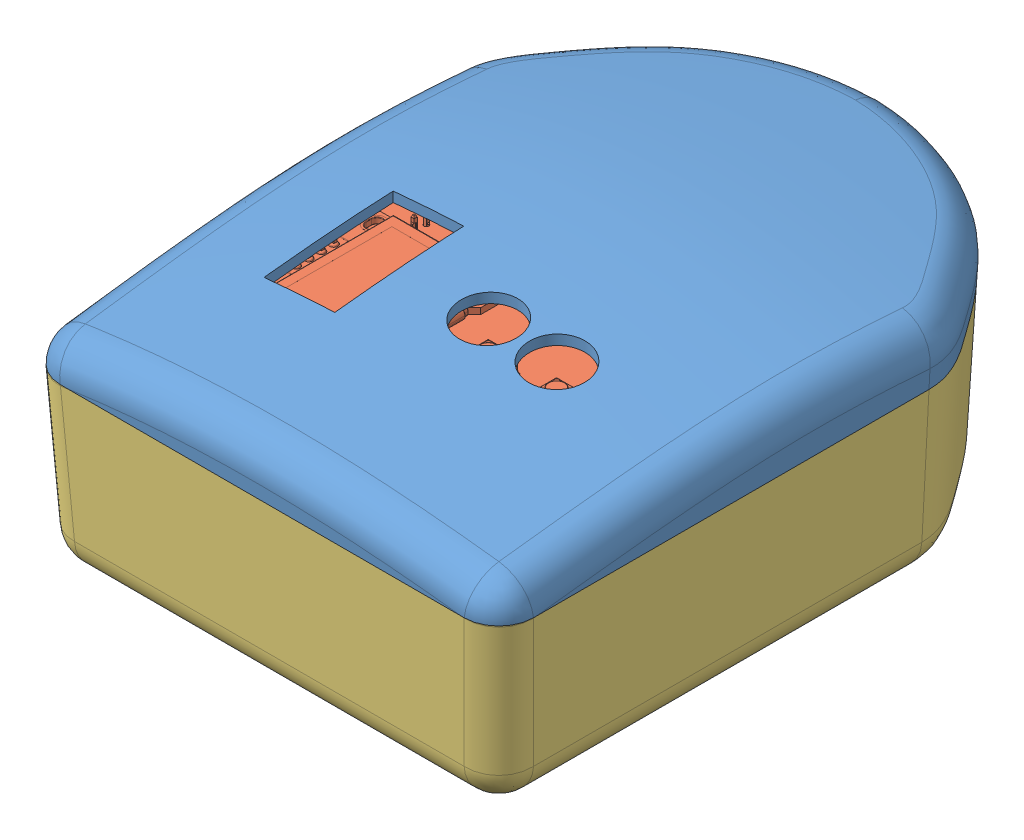
SolidWorks assembly advanced_design_assembly, configuration Default. Lengths in mm.
Overall size (102.14 51.45 130.38).
4 component instances, 4 part files, 2 mates.
Components (placement in the parent):
- Part2^advanced_design_assembly-1: Part2^advanced_design_assembly [Default] at origin (virtual)
- top lid-2: top lid [Default] at (-349.6865 89.9317 499.6127) size (102.14 20.09 130.38)
- fabricated_PCB_v1.step-2: fabricated_PCB_v1.step [Default] at (19.1402 125.1029 129.4245) x (0 0 1) z (0 -1 0) size (61.21 84.93 14.61)
- bottom box-1: bottom box [Default] at (-349.6865 89.9317 499.6127) size (101.09 34.39 128.32)
Mates (geometry in assembly coordinates):
- Coincident1: coincident aligned: line of top lid-2 through (-65.6253 121.9317 198.6672) axis (1 0 0); line of bottom box-1 through (-65.6253 121.9317 198.6672) axis (1 0 0)
- Coincident2: coincident aligned: line of top lid-2 through (21.1676 121.9317 191.1158) axis (0 0 -1); line of bottom box-1 through (21.1676 121.9317 191.1158) axis (0 0 -1)
